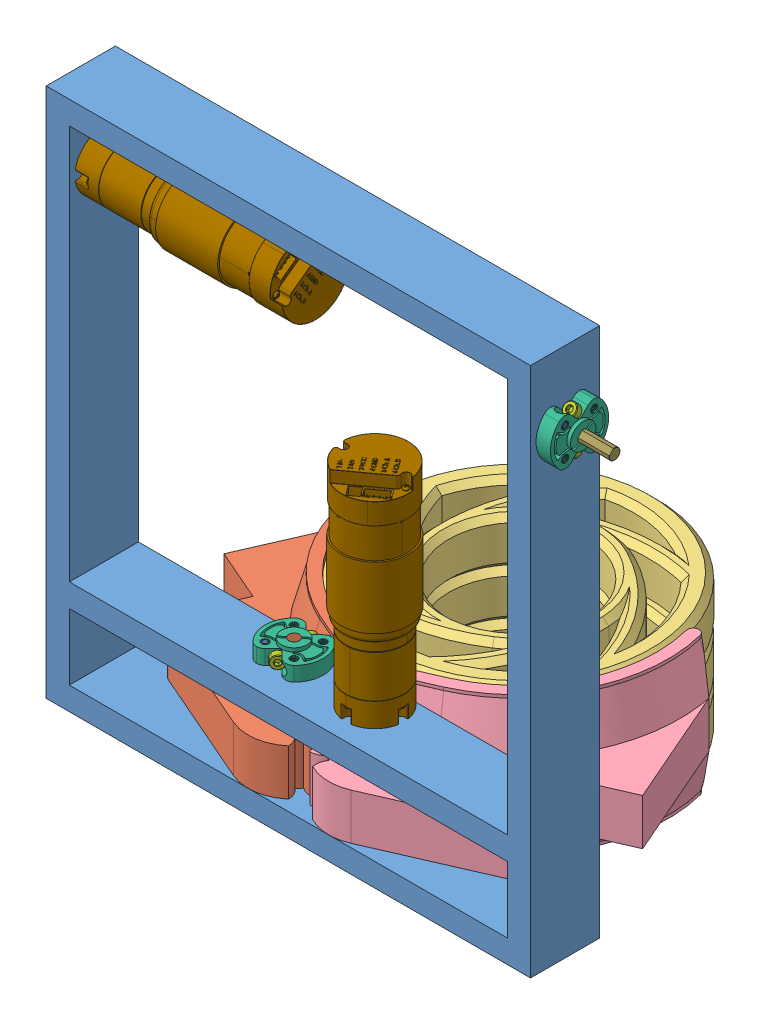
SolidWorks assembly pince, configuration Défaut. Lengths in mm.
Overall size (305.3 304.8 231.96).
35 component instances, 12 part files, 51 mates.
Components (placement in the parent):
- pinceBase-1: pinceBase [Défaut] at (-7.7147 -78.3287 254) size (266.7 292.1 38.1)
- pinceGauche-2: pinceGauche [Défaut] at (-7.7538 -65.6287 146.4997) x (1 0 -0.000386) z (0.000386 0 1) size (118.44 76.2 149.15)
- GP TAKTIK 2025-1: GP TAKTIK 2025 [Défaut] at (-7.7538 -65.6287 146.4997) x (0.997493 0 0.070767) z (-0.070767 0 0.997493) size (152.4 25.41 152.4)
- GP TAKTIK 2025-2: GP TAKTIK 2025 [Défaut] at (-7.7538 -91.0287 146.4997) x (0.999817 0 -0.019129) z (0.019129 0 0.999817) size (152.4 25.41 152.4)
- pinceDroite-5: pinceDroite [Défaut] at (-7.6756 -40.2287 146.4997) x (-1 0 -0.000386) z (-0.000386 0 1) size (117.95 76.2 149.15)
- 1611-0514-0006 Roulement-2: 1611-0514-0006 Roulement [Défaut] at (-29.9397 -45.4287 247.65) x (0.911314 0 -0.411713) z (0.411713 0 0.911314) size (15 5 15)
- 1611-0514-0006 Roulement-5: 1611-0514-0006 Roulement [Défaut] at (-29.9397 -60.4287 247.65) x (-0.666064 0 -0.745895) z (-0.745895 0 0.666064) size (15 5 15)
- 1309-0016-1006 hub-2: 1309-0016-1006 hub [Défaut] at (10.6154 -45.0024 229.8604) x (-0.244752 0 -0.969586) z (0 1 0) size (28.36 32 10.95)
  - 1309-0016-1006 assembly.STEP-1: 1309-0016-1006 assembly.STEP [Défaut] at origin size (28.36 32 10.95)
    - 1309-0016-1006.STEP-1: 1309-0016-1006.STEP [Défaut] at (-18.2019 0.5776 8.7736) size (25.38 32 10)
    - 2800-0004-0014_90128A207.STEP-1: 2800-0004-0014_90128A207.STEP [Défaut] at (-16.149 11.6963 8.7736) x (0.5 -0.5 -0.707107) z (0.707107 0.707107 0) size (7 7 18.01)
    - 2800-0004-0014_90128A207.STEP-2: 2800-0004-0014_90128A207.STEP [Défaut] at (-20.2547 -10.5411 8.7736) x (-0.5 0.5 -0.707107) z (-0.707107 -0.707107 0) size (7 7 18.01)
- 2800-0004-0030-vis-1: 2800-0004-0030-vis [Défaut] at (4.7956 -30.6287 241.8513) x (-0.557574 0 -0.830127) z (0 1 0) size (7 7 34.01)
- 2800-0004-0030-vis-2: 2800-0004-0030-vis [Défaut] at (20.3089 -30.6287 237.9353) x (1 0 0) z (0 1 0) size (7 7 34.01)
- 2800-0004-0030-vis-3: 2800-0004-0030-vis [Défaut] at (8.7116 -30.6287 257.3647) x (1 0 0) z (0 1 0) size (7 7 34.01)
- 2800-0004-0030-vis-4: 2800-0004-0030-vis [Défaut] at (24.225 -30.6287 253.4487) x (1 0 0) z (0 1 0) size (7 7 34.01)
- 5202-0002-0019 Moteur-1: 5202-0002-0019 Moteur [Défaut] at (14.5103 -16.4162 247.65) x (1 0 0) z (0 -1 0) size (37.51 37.5 140.7)
- 5202-0002-0019 Moteur-2: 5202-0002-0019 Moteur [Défaut] at (-128.3647 175.6713 254) x (0 0 1) z (-1 0 0) size (37.51 37.5 140.7)
- 2800-0004-0016-vis16-2: 2800-0004-0016-vis16 [Défaut] at (-120.3022 183.6713 262) x (0 0.768177 -0.640238) z (1 0 0) size (7 7 20.01)
- 2800-0004-0016-vis16-3: 2800-0004-0016-vis16 [Défaut] at (6.5103 -8.3537 255.65) x (0.999049 0 -0.043598) z (0 1 0) size (7 7 20.01)
- 1309-0016-1006 hub-4: 1309-0016-1006 hub [Défaut] at (-30.5173 -21.1899 265.8519) x (0 0 1) z (0 1 0) size (28.36 32 10.95)
  - 1309-0016-1006 assembly.STEP-1: 1309-0016-1006 assembly.STEP [Défaut] at origin size (28.36 32 10.95)
    - 1309-0016-1006.STEP-1: 1309-0016-1006.STEP [Défaut] at (-18.2019 0.5776 8.7736) size (25.38 32 10)
    - 2800-0004-0014_90128A207.STEP-1: 2800-0004-0014_90128A207.STEP [Défaut] at (-16.149 11.6963 8.7736) x (0.5 -0.5 -0.707107) z (0.707107 0.707107 0) size (7 7 18.01)
    - 2800-0004-0014_90128A207.STEP-2: 2800-0004-0014_90128A207.STEP [Défaut] at (-20.2547 -10.5411 8.7736) x (-0.5 0.5 -0.707107) z (-0.707107 -0.707107 0) size (7 7 18.01)
- 2800-0004-0016-vis16-5: 2800-0004-0016-vis16 [Défaut] at (-37.9397 -8.3537 255.65) x (-0.867773 0 -0.49696) z (0 1 0) size (7 7 20.01)
- axeBasePince-1: axeBasePince [Défaut] at (-29.9397 -6.4162 247.65) x (1 0 0) z (0 -1 0) size (6 6 69.85)
- 1309-0016-1006 hub-5: 1309-0016-1006 hub [Défaut] at (120.8616 193.8731 253.4224) x (0 1 0) z (1 0 0) size (28.36 32 10.95)
  - 1309-0016-1006 assembly.STEP-1: 1309-0016-1006 assembly.STEP [Défaut] at origin size (28.36 32 10.95)
    - 1309-0016-1006.STEP-1: 1309-0016-1006.STEP [Défaut] at (-18.2019 0.5776 8.7736) size (25.38 32 10)
    - 2800-0004-0014_90128A207.STEP-1: 2800-0004-0014_90128A207.STEP [Défaut] at (-16.149 11.6963 8.7736) x (0.5 -0.5 -0.707107) z (0.707107 0.707107 0) size (7 7 18.01)
    - 2800-0004-0014_90128A207.STEP-2: 2800-0004-0014_90128A207.STEP [Défaut] at (-20.2547 -10.5411 8.7736) x (-0.5 0.5 -0.707107) z (-0.707107 -0.707107 0) size (7 7 18.01)
- 2800-0004-0016-vis16-6: 2800-0004-0016-vis16 [Défaut] at (133.6978 183.6713 262) x (0 -0.817303 0.576209) z (1 0 0) size (7 7 20.01)
- 2101-0006-0040-D-1: 2101-0006-0040-D [Défaut] at (152.9353 175.6713 254) x (0 -0.707107 0.707107) z (0 -0.707107 -0.707107) size (6 40 5.5)
- GP TAKTIK 2025-3: GP TAKTIK 2025 [Défaut] at (-7.7538 -40.2287 146.4997) x (0.543235 0 0.839581) z (-0.839581 0 0.543235) size (152.4 25.41 152.4)
Mates (geometry in assembly coordinates):
- Coaxiale2: concentric: circle of pinceBase-1; circle of pinceGauche-2
- Coïncidente4: coincident: plane of pinceBase-1 through (-7.7147 -65.6287 254) normal (0 1 0); plane of pinceGauche-2 through (-7.7538 -65.6287 146.4997) normal (0 -1 0)
- Coïncidente7: coincident: plane of pinceGauche-2 through (-7.7538 -65.6287 146.4997) normal (0 -1 0); plane of GP TAKTIK 2025-1 through (-7.7538 -65.6287 146.4997) normal (0 -1 0)
- Coaxiale4: concentric: cylinder of pinceGauche-2 through (-7.7538 -40.2287 146.4997) axis (0 -1 0) radius 76.2; cylinder of GP TAKTIK 2025-1 through (-7.7538 -65.6287 146.4997) axis (0 1 0) radius 76.2
- Coaxiale5: concentric: cylinder of GP TAKTIK 2025-1 through (-7.7538 -65.6287 146.4997) axis (0 1 0) radius 76.2; cylinder of GP TAKTIK 2025-2 through (-7.7538 -91.0287 146.4997) axis (0 1 0) radius 76.2
- Coïncidente8: coincident: plane of GP TAKTIK 2025-1 through (-7.7538 -65.6287 146.4997) normal (0 -1 0); plane of GP TAKTIK 2025-2 through (-7.7538 -65.6287 146.4997) normal (0 1 0)
- Coaxiale6: concentric: circle of pinceBase-1; cylinder of pinceDroite-5 through (14.5103 -61.2287 247.65) axis (0 -1 0) radius 3.175
- Coïncidente10: coincident: plane of pinceBase-1 through (-7.7147 -65.6287 254) normal (0 1 0); plane of pinceDroite-5 through (-7.6756 -65.6287 146.4997) normal (0 -1 0)
- Coaxiale7: concentric: cylinder of pinceGauche-2 through (-29.9397 -91.0287 247.65) axis (0 1 0) radius 7.2; cylinder of 1611-0514-0006 Roulement-2 through (-29.9397 -41.4287 247.65) axis (0 -1 0) radius 7
- Coïncidente14: coincident: plane of pinceGauche-2 through (-29.9397 -41.4287 247.65) normal (0 1 0); plane of 1611-0514-0006 Roulement-2 through (-29.9397 -41.4287 247.65) normal (0 -1 0)
- Coaxiale10: concentric: cylinder of pinceGauche-2 through (-29.9397 -91.0287 247.65) axis (0 1 0) radius 7.2; cylinder of 1611-0514-0006 Roulement-5 through (-29.9397 -64.4287 247.65) axis (0 1 0) radius 7
- Coïncidente18: coincident: plane of pinceGauche-2 through (-29.9397 -64.4287 247.65) normal (0 -1 0); plane of 1611-0514-0006 Roulement-5 through (-29.9397 -64.4287 247.65) normal (0 1 0)
- Coïncidente19: coincident: plane of pinceDroite-5 through (-7.6756 -40.2287 146.4997) normal (0 1 0); plane of 1309-0016-1006 hub-2/1309-0016-1006 assembly.STEP-1/1309-0016-1006.STEP-1 through (14.5103 -40.2287 247.65) normal (0 -1 0)
- Coaxiale11: concentric: cylinder of pinceDroite-5 through (14.5103 -61.2287 247.65) axis (0 -1 0) radius 3.175; cylinder of 1309-0016-1006 hub-2/1309-0016-1006 assembly.STEP-1/1309-0016-1006.STEP-1 through (14.5103 -40.4792 247.65) axis (0 1 0) radius 3
- Coaxiale12: concentric: cylinder of pinceDroite-5 through (20.3089 -91.0287 237.9353) axis (0 1 0) radius 2.2; circle of 1309-0016-1006 hub-2/1309-0016-1006 assembly.STEP-1/1309-0016-1006.STEP-1
- Coaxiale14: concentric: cylinder of pinceDroite-5 through (24.225 -60.6287 253.4487) axis (0 -1 0) radius 3.7; cylinder of 2800-0004-0030-vis-4 through (24.225 -64.6287 253.4487) axis (0 1 0) radius 3.5
- Coïncidente22: coincident: plane of pinceDroite-5 through (24.225 -60.6287 253.4487) normal (0 -1 0); plane of 2800-0004-0030-vis-4 through (24.225 -60.6287 253.4487) normal (0 1 0)
- Coaxiale15: concentric: cylinder of pinceDroite-5 through (8.7116 -60.6287 257.3647) axis (0 -1 0) radius 3.7; cylinder of 2800-0004-0030-vis-3 through (8.7116 -64.6287 257.3647) axis (0 1 0) radius 3.5
- Coïncidente23: coincident: plane of pinceDroite-5 through (8.7116 -60.6287 257.3647) normal (0 -1 0); plane of 2800-0004-0030-vis-3 through (8.7116 -60.6287 257.3647) normal (0 1 0)
- Coaxiale16: concentric: cylinder of pinceDroite-5 through (20.3089 -60.6287 237.9353) axis (0 -1 0) radius 3.7; cylinder of 2800-0004-0030-vis-2 through (20.3089 -64.6287 237.9353) axis (0 1 0) radius 3.5
- Coïncidente24: coincident: plane of pinceDroite-5 through (20.3089 -60.6287 237.9353) normal (0 -1 0); plane of 2800-0004-0030-vis-2 through (20.3089 -60.6287 237.9353) normal (0 1 0)
- Coaxiale17: concentric: cylinder of pinceDroite-5 through (4.7956 -60.6287 241.8513) axis (0 -1 0) radius 3.7; cylinder of 2800-0004-0030-vis-1 through (4.7956 -64.6287 241.8513) axis (0 1 0) radius 3.5
- Coïncidente25: coincident: plane of pinceDroite-5 through (4.7956 -60.6287 241.8513) normal (0 -1 0); plane of 2800-0004-0030-vis-1 through (4.7956 -60.6287 241.8513) normal (0 1 0)
- Coaxiale18: concentric: cylinder of 1309-0016-1006 hub-2/1309-0016-1006 assembly.STEP-1/1309-0016-1006.STEP-1 through (14.5103 -40.4792 247.65) axis (0 1 0) radius 3; cylinder of 5202-0002-0019 Moteur-1 through (14.5103 -40.4162 247.65) axis (0 1 0) radius 3
- Coïncidente28: coincident: plane of pinceBase-1 through (125.6373 -16.4162 234.95) normal (0 1 0); plane of 5202-0002-0019 Moteur-1 through (14.5103 -16.4162 247.65) normal (0 -1 0)
- Coaxiale19: concentric: cylinder of pinceBase-1 through (125.6353 175.6713 254) axis (-1 0 0) radius 3.175; cylinder of 5202-0002-0019 Moteur-2 through (-152.3647 175.6713 254) axis (1 0 0) radius 3
- Coïncidente29: coincident: plane of pinceBase-1 through (-128.3647 213.7713 234.95) normal (1 0 0); plane of 5202-0002-0019 Moteur-2 through (-128.3647 175.6713 254) normal (-1 0 0)
- Coaxiale22: concentric: cylinder of pinceBase-1 through (125.6353 183.6713 262) axis (-1 0 0) radius 2; circle of 5202-0002-0019 Moteur-2
- Coaxiale29: concentric: cylinder of pinceBase-1 through (-136.3022 183.6713 262) axis (-1 0 0) radius 4.7625; cylinder of 2800-0004-0016-vis16-2 through (-140.3022 183.6713 262) axis (1 0 0) radius 3.5
- Coïncidente39: coincident: plane of pinceBase-1 through (-136.3022 183.6713 262) normal (-1 0 0); plane of 2800-0004-0016-vis16-2 through (-136.3022 183.6713 262) normal (1 0 0)
- Coaxiale30: concentric: cylinder of pinceBase-1 through (22.5103 -24.3537 255.65) axis (0 -1 0) radius 3.9688; circle of 5202-0002-0019 Moteur-1
- Coaxiale31: concentric: circle of pinceBase-1; cylinder of 2800-0004-0016-vis16-3 through (6.5103 -28.3537 255.65) axis (0 1 0) radius 3.5
- Coïncidente40: coincident: plane of pinceBase-1 through (6.5103 -24.3537 255.65) normal (0 -1 0); plane of 2800-0004-0016-vis16-3 through (6.5103 -24.3537 255.65) normal (0 1 0)
- Coaxiale32: concentric: cylinder of pinceBase-1 through (-29.9397 -2.1287 247.65) axis (0 -1 0) radius 3.175; cylinder of 1309-0016-1006 hub-4/1309-0016-1006 assembly.STEP-1/1309-0016-1006.STEP-1 through (-29.9397 -16.6667 247.65) axis (0 1 0) radius 3
- Coaxiale33: concentric: cylinder of pinceBase-1 through (-37.9397 -41.8162 255.65) axis (0 1 0) radius 2; circle of 1309-0016-1006 hub-4/1309-0016-1006 assembly.STEP-1/1309-0016-1006.STEP-1
- Coïncidente42: coincident: plane of pinceBase-1 through (125.6373 -16.4162 234.95) normal (0 1 0); plane of 1309-0016-1006 hub-4/1309-0016-1006 assembly.STEP-1/1309-0016-1006.STEP-1 through (-29.9397 -16.4162 247.65) normal (0 -1 0)
- Coaxiale34: concentric: cylinder of pinceBase-1 through (-37.9397 -24.3537 255.65) axis (0 -1 0) radius 3.9688; cylinder of 2800-0004-0016-vis16-5 through (-37.9397 -28.3537 255.65) axis (0 1 0) radius 3.5
- Coïncidente43: coincident: plane of pinceBase-1 through (-37.9397 -24.3537 255.65) normal (0 -1 0); plane of 2800-0004-0016-vis16-5 through (-37.9397 -24.3537 255.65) normal (0 1 0)
- Coaxiale35: concentric: cylinder of 1309-0016-1006 hub-4/1309-0016-1006 assembly.STEP-1/1309-0016-1006.STEP-1 through (-29.9397 -16.6667 247.65) axis (0 1 0) radius 3; cylinder of axeBasePince-1 through (-29.9397 -76.2662 247.65) axis (0 1 0) radius 3
- Coïncidente44: coincident: plane of 1309-0016-1006 hub-4/1309-0016-1006 assembly.STEP-1/1309-0016-1006.STEP-1 through (-29.9397 -6.4162 247.65) normal (0 1 0); plane of axeBasePince-1 through (-29.9397 -6.4162 247.65) normal (0 1 0)
- Contr.Engrenages1: gear = 25.4 : 25.4 mm: circle of pinceDroite-5; circle of pinceGauche-2
- Coïncidente45: coincident: plane of pinceBase-1 through (125.6353 -65.6287 234.95) normal (1 0 0); plane of 1309-0016-1006 hub-5/1309-0016-1006 assembly.STEP-1/1309-0016-1006.STEP-1 through (125.6353 175.6713 254) normal (-1 0 0)
- Coaxiale36: concentric: circle of pinceBase-1; circle of 1309-0016-1006 hub-5/1309-0016-1006 assembly.STEP-1/1309-0016-1006.STEP-1
- Coaxiale37: concentric: circle of pinceBase-1; circle of 1309-0016-1006 hub-5/1309-0016-1006 assembly.STEP-1/1309-0016-1006.STEP-1
- Coaxiale38: concentric: cylinder of pinceBase-1 through (125.6353 183.6713 262) axis (-1 0 0) radius 2; cylinder of 2800-0004-0016-vis16-6 through (113.6978 183.6713 262) axis (1 0 0) radius 3.5
- Coïncidente49: coincident: plane of pinceBase-1 through (117.6978 183.6713 262) normal (-1 0 0); plane of 2800-0004-0016-vis16-6 through (117.6978 183.6713 262) normal (1 0 0)
- Coaxiale40: concentric: cylinder of 1309-0016-1006 hub-5/1309-0016-1006 assembly.STEP-1/1309-0016-1006.STEP-1 through (125.3848 175.6713 254) axis (1 0 0) radius 3; cylinder of 2101-0006-0040-D-1 through (112.9353 175.6713 254) axis (1 0 0) radius 3
- Parallèle1: parallel: plane of 1309-0016-1006 hub-5/1309-0016-1006 assembly.STEP-1/1309-0016-1006.STEP-1 through (125.3848 177.4249 255.7536) normal (0 -0.707107 -0.707107); plane of 2101-0006-0040-D-1 through (112.9353 177.439 255.7678) normal (0 0.707107 0.707107)
- Coïncidente54: coincident: plane of pinceBase-1 through (112.9353 213.7713 234.95) normal (-1 0 0); plane of 2101-0006-0040-D-1 through (112.9353 175.6713 254) normal (-1 0 0)
- Coaxiale41: concentric: cylinder of GP TAKTIK 2025-1 through (-7.7538 -65.6287 146.4997) axis (0 1 0) radius 38.1; cylinder of GP TAKTIK 2025-3 through (-7.7538 -40.2287 146.4997) axis (0 1 0) radius 38.1
- Coïncidente55: coincident: plane of GP TAKTIK 2025-1 through (-7.7538 -40.2287 146.4997) normal (0 1 0); plane of GP TAKTIK 2025-3 through (-7.7538 -40.2287 146.4997) normal (0 -1 0)
